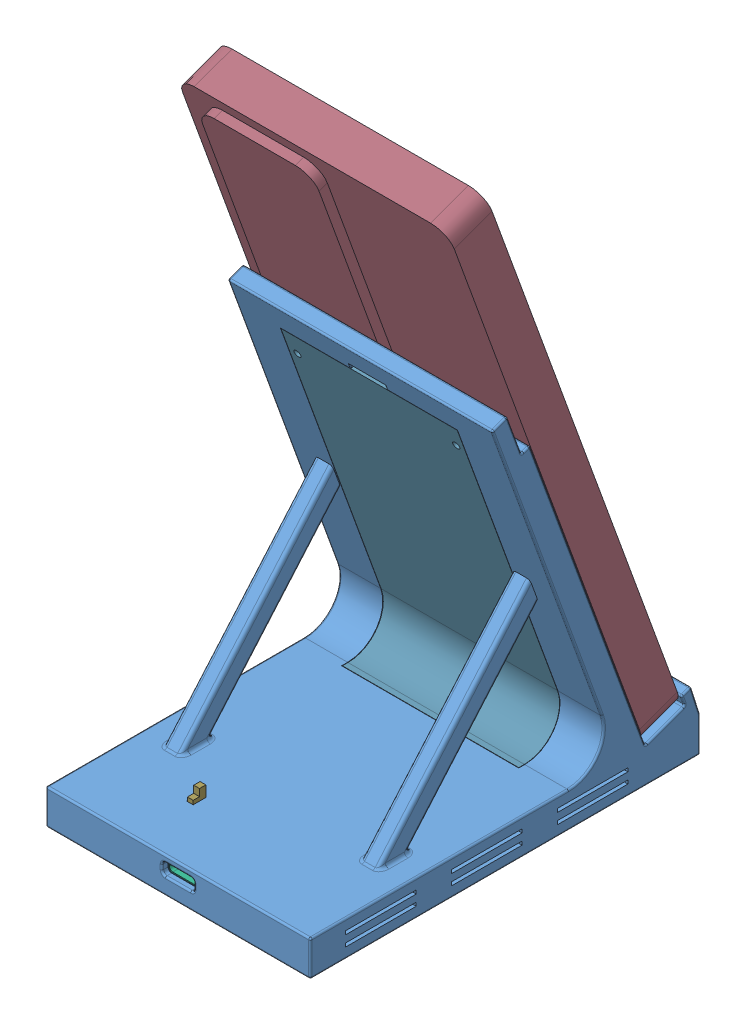
SolidWorks assembly P60支架装配体_配重块, configuration 默认. Lengths in mm.
Overall size (77 167.54 112.5).
31 component instances, 16 part files, 20 mates.
Components (placement in the parent):
- P60支架-1: P60支架 [默认] at (932.5062 0 -1183.2093) size (75 110.1 110.5)
- 嘉立创配重块-1: 嘉立创配重块 [默认] at (932.5062 1.5 -1183.2093) x (1 0 0) z (0 1 0) size (60 80 1.6)
- 充电线圈-1: 充电线圈 [默认] at (932.5062 78.5713 -1193.5075) x (1 0 0) z (0 -0.939693 -0.34202) size (43 1.52 55.03)
- 充电零件板-1: 充电零件板 [默认] at (932.5062 3.64 -1178.9215) x (-1 0 0) z (0 0 -1) size (21 2 28)
- TypeC电路板-2: TypeC电路板 [默认] at (954.5033 3.6 -1126.71) x (0 0 -1) z (0 1 0) size (30 34.97 13.16)
  - TypeC电路板.STEP-1: TypeC电路板.STEP [默认] at origin size (30 34.97 13.16)
    - TypeC______.STEP.STEP-1: TypeC______.STEP.STEP [默认] at origin size (30 34.97 13.16)
      - 5v06-R1.STEP.STEP-1: 5v06-R1.STEP.STEP [默认] at (25.0953 30.8357 1.2) x (-1 0 0) z (0 0 1) size (2 1.3 0.61)
        - R0805.STEP.STEP-1: R0805.STEP.STEP [默认] at origin size (2 1.3 0.61)
          - COMPOUND.STEP.STEP-1: COMPOUND.STEP.STEP [默认] at origin size (2 1.3 0.61)
      - 5v06-USB1.STEP.STEP-1: 5v06-USB1.STEP.STEP [默认] at (8.1992 21.9972 1.2) x (0 -1 0) z (0 0 1) size (8.95 7.58 4.16)
        - USB-C-SMD_TYPE-C-6PIN-2MD-073.STEP.STEP-1: USB-C-SMD_TYPE-C-6PIN-2MD-073.STEP.STEP [默认] at origin size (8.95 7.58 4.16)
          - COMPOUND-1.STEP.STEP-1: COMPOUND-1.STEP.STEP [默认] at origin size (8.95 7.58 4.16)
      - 5v06-U2.STEP.STEP-1: 5v06-U2.STEP.STEP [默认] at (19.685 34.9251 0) x (-1 0 0) z (0 0 -1) size (8.51 3.81 11.5) (hidden)
        - SW-TH_DEALON_SS-12D01-GX.STEP.STEP-1: SW-TH_DEALON_SS-12D01-GX.STEP.STEP [默认] at origin size (8.51 3.81 11.5)
          - COMPOUND-2.STEP.STEP-1: COMPOUND-2.STEP.STEP [默认] at origin size (8.51 3.81 11.5)
      - 5v06-C1.STEP.STEP-1: 5v06-C1.STEP.STEP [默认] at (18.2118 28.8799 1.2) size (3.2 2.52 0.9)
        - C1210.STEP.STEP-1: C1210.STEP.STEP [默认] at origin size (3.2 2.52 0.9)
          - SOLID-3.STEP.STEP-1: SOLID-3.STEP.STEP [默认] at origin size (3.2 2.52 0.9)
      - 5v06-C2.STEP.STEP-1: 5v06-C2.STEP.STEP [默认] at (24.13 13.843 1.2) x (0 1 0) z (0 0 1) size (1.6 0.8 0.8)
        - C0603.STEP.STEP-1: C0603.STEP.STEP [默认] at origin size (1.6 0.8 0.8)
          - SOLID-4.STEP.STEP-1: SOLID-4.STEP.STEP [默认] at origin size (1.6 0.8 0.8)
      - 5v06-U4.STEP.STEP-1: 5v06-U4.STEP.STEP [默认] at (18.386 14.645 1.2) size (4.1 4.3 1.61)
        - SOT-89-3_L4.5-W2.5-P1.50-LS4.2-BR.STEP.STEP-1: SOT-89-3_L4.5-W2.5-P1.50-LS4.2-BR.STEP.STEP [默认] at origin size (4.1 4.3 1.61)
          - SOLID-5.STEP.STEP-1: SOLID-5.STEP.STEP [默认] at origin size (4.1 4.3 1.61)
      - Board.STEP.STEP-1: Board.STEP.STEP [默认] at origin size (29.97 34.97 1.2)
- Led5mmRojo_.step-1: Led5mmRojo_.step [默认] at (932.5062 4.75 -1215.2093) x (0 0 -1) z (-0.050369 0.998731 0) size (25.5 5.8 5.4)
- 开关-1: 开关 [默认] at (919.5689 5 -1146.3969) x (0 0 1) z (-1 0 0) size (8.5 11.2 3.5)
- P60手机-1: P60手机 [默认] at (931.5062 86.8199 -1195.2491) x (-1 0 0) z (0 0.34202 -0.939693) size (77 163.5 13.9)
- P60线圈支架零件-1: P60线圈支架零件 [默认] at (932.5062 3.0953 -1170.6808) x (0 0 -1) z (1 0 0) size (32.03 95.56 50)
- P60底板-1: P60底板 [默认] at (916.4579 0 -1186.0237) x (0 0 -1) z (1 0 0) size (102.06 4.25 64.8)
Mates (geometry in assembly coordinates):
- 重合68: coincident anti-aligned: plane of P60支架-1 through (932.5062 0 -1183.2093) normal (0 -1 0)
- 同心2: concentric aligned: cylinder of Led5mmRojo_.step-1 through (932.5062 4.75 -1233.2093) axis (0 0 -1) radius 2.5; cylinder of P60支架-1 through (932.5062 4.75 -1224.8553) axis (0 0 -1) radius 2.6
- 重合75: coincident aligned: plane of Led5mmRojo_.step-1 through (932.4961 4.9497 -1232.2093) normal (0 0 1); plane of P60支架-1 through (-399067.4938 -0.001 -1232.2093) normal (0 0 1)
- 宽度31: width anti-aligned: plane of TypeC电路板-2/TypeC电路板.STEP-1/TypeC______.STEP.STEP-1/Board.STEP.STEP-1 through (938.4935 3.6 -1137.4342) normal (1 0 0); plane of P60支架-1 through (926.5189 3.6 -1129.9469) normal (-1 0 0); plane of TypeC电路板-2/TypeC电路板.STEP-1/TypeC______.STEP.STEP-1/Board.STEP.STEP-1 through (938.5935 -0.001 290361.0407) normal (-1 0 0); plane of P60支架-1 through (926.4189 -0.001 290361.0407) normal (1 0 0)
- 重合76: coincident anti-aligned: plane of TypeC电路板-2/TypeC电路板.STEP-1/TypeC______.STEP.STEP-1/Board.STEP.STEP-1 through (938.4935 3.6 -1129.9469) normal (0 0 1); plane of P60支架-1 through (-399067.4938 -0.001 -1129.9469) normal (0 0 -1)
- 重合77: coincident anti-aligned: plane of P60支架-1 through (1080.051 111.0961 -1186.4133) normal (0 0.34202 -0.939693); plane of P60手机-1 through (931.5062 86.8199 -1195.2491) normal (0 -0.34202 0.939693)
- 重合78: coincident aligned: plane of P60支架-1 through (970.0062 10 -1128.2093) normal (1 0 0); plane of P60手机-1 through (970.0062 167.5388 -1178.0015) normal (1 0 0)
- 重合79: coincident anti-aligned: plane of P60支架-1 through (871.3165 10 -1223.2093) normal (0 0.939693 0.34202); plane of P60手机-1 through (970.0062 13.899 -1233.9218) normal (0 -0.939693 -0.34202)
- 同心3: concentric aligned: cylinder of 充电线圈-1 through (932.5062 78.0583 -1192.098) axis (0 0.34202 -0.939693) radius 21.5; cylinder of P60线圈支架零件-1 through (932.5062 78.078 -1192.1522) axis (0 0.34202 -0.939693) radius 22
- 重合82: coincident aligned: plane of P60支架-1 through (1080.051 10 -1215.6536) normal (0 -0.34202 0.939693); plane of P60线圈支架零件-1 through (957.5062 23.4202 -1210.769) normal (0 -0.34202 0.939693)
- 宽度32: width anti-aligned: plane of P60支架-1 through (907.4062 20 -1201.3721) normal (1 0 0); plane of P60线圈支架零件-1 through (957.6062 20 -1201.3721) normal (-1 0 0); plane of P60支架-1 through (907.5062 20 -1201.3721) normal (-1 0 0); plane of P60线圈支架零件-1 through (957.5062 20 -1201.3721) normal (1 0 0)
- 距离6: distance = 0.1 mm anti-aligned: plane of P60线圈支架零件-1 through (957.5062 101.5358 -1182.3373) normal (0 0.939693 0.34202); plane of P60支架-1 through (907.4062 -162564.6059 445739.5065) normal (0 -0.939693 -0.34202)
- 重合83: coincident aligned: plane of P60支架-1 through (932.5062 0 -1183.2093) normal (0 -1 0); plane of P60底板-1 through (916.4579 0 -1186.0237) normal (0 -1 0)
- 宽度33: width anti-aligned: plane of P60支架-1 through (900.0062 -0.001 290361.0407) normal (1 0 0); plane of P60底板-1 through (965.0062 -0.001 290361.0407) normal (-1 0 0); plane of P60支架-1 through (900.1062 1.5 -1134.3093) normal (-1 0 0); plane of P60底板-1 through (964.9062 1.5 -1134.3093) normal (1 0 0)
- 宽度34: width anti-aligned: plane of P60支架-1 through (-399067.4938 -0.001 -1232.2093) normal (0 0 1); plane of P60底板-1 through (-399067.4938 -0.001 -1134.2093) normal (0 0 -1); plane of P60支架-1 through (900.1062 1.5 -1232.1093) normal (0 0 -1); plane of P60底板-1 through (900.1062 1.5 -1134.3093) normal (0 0 1)
- 宽度35: width anti-aligned: plane of P60支架-1 through (900.0062 -0.001 290361.0407) normal (1 0 0); plane of P60支架-1 through (965.0062 -0.001 290361.0407) normal (-1 0 0); plane of 嘉立创配重块-1 through (902.5062 3.1 -1143.2093) normal (-1 0 0); plane of 嘉立创配重块-1 through (962.5062 3.1 -1143.2093) normal (1 0 0)
- 宽度36: width anti-aligned: plane of P60支架-1 through (-399067.4938 -0.001 -1134.2093) normal (0 0 -1); plane of P60支架-1 through (-399067.4938 -0.001 -1232.2093) normal (0 0 1); plane of 嘉立创配重块-1 through (902.5062 3.1 -1143.2093) normal (0 0 1); plane of 嘉立创配重块-1 through (902.5062 3.1 -1223.2093) normal (0 0 -1)
- 重合84: coincident anti-aligned: plane of 嘉立创配重块-1 through (932.5062 1.5 -1183.2093) normal (0 -1 0); plane of P60底板-1 through (916.4579 1.5 -1186.0237) normal (0 1 0)
- 重合85: coincident anti-aligned: plane of P60支架-1 through (932.5062 9 -1183.2093) normal (0 -1 0); plane of 开关-1 through (919.5689 9 -1146.3969) normal (0 1 0)
- 距离8: distance = 0.2 mm anti-aligned: plane of TypeC电路板-2/TypeC电路板.STEP-1/TypeC______.STEP.STEP-1/Board.STEP.STEP-1 through (932.5062 4.8 -1146.263) normal (0 1 0); plane of 开关-1 through (919.5689 5 -1146.3969) normal (0 -1 0)
